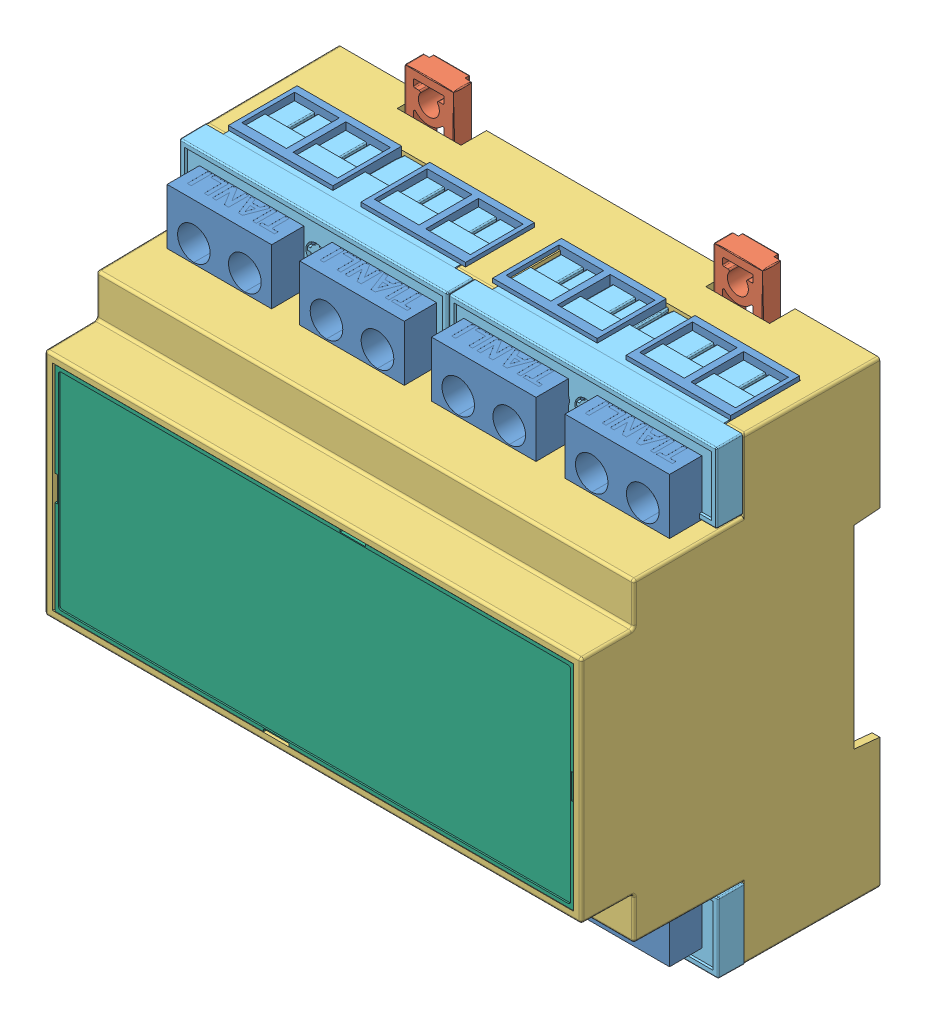
SolidWorks assembly Трехфазный счетчик, сборка, configuration Default. Lengths in mm.
Overall size (107.09 109.14 58.07).
12 component instances, 7 part files, 5 mates.
Components (placement in the parent):
- THREE_PHASE_METER___.step-1: THREE_PHASE_METER___.step [Default] at (-33.1626 -34.0651 0) x (1 0 0) z (0 0 1) size (106.55 91.61 40.32)
- CNMB-6-KIT.STEP-1: CNMB-6-KIT.STEP [Default] at (0 19.6482 -28.9579) x (0 -1 0) z (0 0 1) size (109.14 106.24 58.15)
  - CNMB-6-Base-1.STEP-1: CNMB-6-Base-1.STEP [Default] at (72.4133 -37.4776 -1.5362) x (0 0 -1) z (-1 0 0) size (10.08 104.2 91.1) (hidden)
  - CNMB-CW-1.STEP-1: CNMB-CW-1.STEP [Default] at (-24.9867 28.2255 -1.5211) x (-1 0 0) z (0 0 -1) size (31.75 10.57 6.05)
  - CNMB-6-2-Top-1.STEP-1: CNMB-6-2-Top-1.STEP [Default] at (-16.7867 -11.8228 16.8903) size (90 106.24 58.07)
  - CNMB-CW-1.STEP-2: CNMB-CW-1.STEP [Default] at (-25 -32.3717 -1.5388) x (-1 0 0) z (0 0 -1) size (31.75 10.57 6.05)
  - CNMB-CB-1.STEP-1: CNMB-CB-1.STEP [Default] at (83.5178 31.9408 -1.341) x (1 0 0) z (0 0 -1) size (33.1 11.85 5.73)
  - CNMB-3-TG508P.STEP-1: CNMB-3-TG508P.STEP [Default] at (73.2133 67.9724 24.8638) x (0 0 1) z (1 0 0) size (19.8 52.6 14.8)
  - CNMB-3-TG508P.STEP-2: CNMB-3-TG508P.STEP [Default] at (-16.7867 15.692 24.8638) x (0 0 1) z (-1 0 0) size (19.8 52.6 14.8)
  - CNMB-3-TG508P.STEP-3: CNMB-3-TG508P.STEP [Default] at (73.2133 15.2224 24.8638) x (0 0 1) z (1 0 0) size (19.8 52.6 14.8)
  - CNMB-3-TG508P.STEP-4: CNMB-3-TG508P.STEP [Default] at (-16.7867 -37.058 24.8638) x (0 0 1) z (-1 0 0) size (19.8 52.6 14.8)
  - CNMB-6-PG.STEP-1: CNMB-6-PG.STEP [Default] at (12.0136 -4.007 53.9638) size (42.3 102.2 5.1)
Mates (geometry in assembly coordinates):
- Coincident1: coincident aligned: plane of THREE_PHASE_METER___.step-1 through (-33.1626 -34.0651 0) normal (0 0 1)
- Parallel1: parallel aligned: plane of THREE_PHASE_METER___.step-1 through (-33.1626 -34.0651 0) normal (0 0 1); plane of CNMB-6-KIT.STEP-1/CNMB-6-PG.STEP-1 through (-4.007 7.6347 27.1059) normal (0 0 1)
- Coincident4: coincident aligned: plane of CNMB-6-KIT.STEP-1 through (0 19.6482 -28.9579) normal (1 0 0)
- Width2: width anti-aligned: plane of THREE_PHASE_METER___.step-1 through (-35.7026 -51.5651 -25.0914) normal (-1 0 0); plane of CNMB-6-KIT.STEP-1/CNMB-3-TG508P.STEP-3 through (66.2974 34.4349 -25.0914) normal (1 0 0); plane of THREE_PHASE_METER___.step-1 through (-37.3776 22.6349 -4.0941) normal (-0.999962 0 0.008727); plane of CNMB-6-KIT.STEP-1/CNMB-3-TG508P.STEP-1 through (67.9724 36.4349 -4.0941) normal (0.999962 0 0.008727)
- Width3: width anti-aligned: plane of THREE_PHASE_METER___.step-1 through (-35.7026 34.4349 -25.0914) normal (0 1 0); plane of CNMB-6-KIT.STEP-1/CNMB-3-TG508P.STEP-1 through (66.2974 -51.5651 -25.0914) normal (0 -1 0); plane of THREE_PHASE_METER___.step-1 through (15.3724 36.4349 -4.0941) normal (0 0.999962 0.008727); plane of CNMB-6-KIT.STEP-1/CNMB-3-TG508P.STEP-2 through (68.292 -53.5651 -4.0941) normal (0 -0.999962 0.008727)
